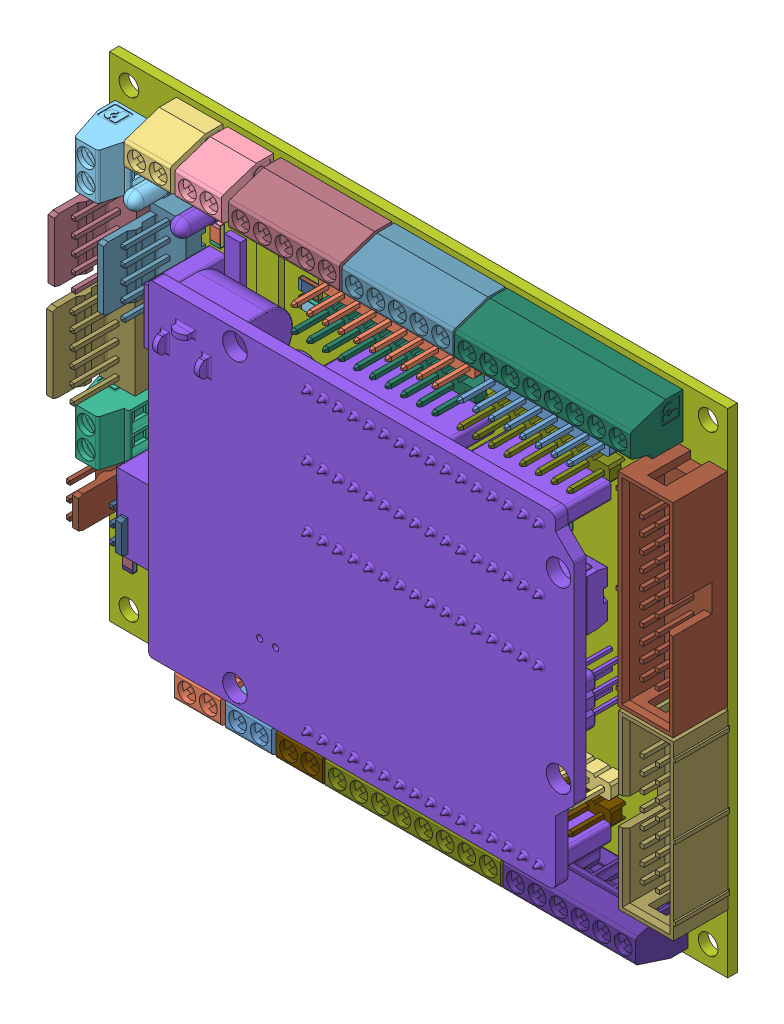
SolidWorks assembly Arduino Uno shield with Uno, configuration Standard. Lengths in mm.
Overall size (100.65 80.01 17.78).
190 component instances, 188 part files, 4 mates.
Components (placement in the parent):
- PPP5f08ec48b7509.stp-1: PPP5f08ec48b7509.stp [Standard] at origin size (100.65 80.01 15.26)
  - CAPRR500W50L750T250H650P002.stp-1: CAPRR500W50L750T250H650P002.stp [Standard] at (21.59 34.29 1.57) x (0 -1 0) z (0 0 1) size (7.5 2.5 6.5)
  - CAPRR500W50L750T250H650P001.stp-1: CAPRR500W50L750T250H650P001.stp [Standard] at (21.59 34.29 1.57) x (0 -1 0) z (0 0 1) size (0.5 0.5 6.5)
  - CAPRR500W50L750T250H650P.stp-1: CAPRR500W50L750T250H650P.stp [Standard] at (21.59 34.29 1.57) x (0 -1 0) z (0 0 1) size (0.5 0.5 6.5)
  - CAPRR500W50L750T250H650P003.stp-1: CAPRR500W50L750T250H650P003.stp [Standard] at (20.32 26.67 1.57) x (0 -1 0) z (0 0 1) size (7.5 2.5 6.5)
  - CAPRR500W50L750T250H650P004.stp-1: CAPRR500W50L750T250H650P004.stp [Standard] at (20.32 26.67 1.57) x (0 -1 0) z (0 0 1) size (0.5 0.5 6.5)
  - CAPRR500W50L750T250H650P005.stp-1: CAPRR500W50L750T250H650P005.stp [Standard] at (20.32 26.67 1.57) x (0 -1 0) z (0 0 1) size (0.5 0.5 6.5)
  - Component_1.stp-1: Component_1.stp [Standard] at (26.67 60.325 1.57) x (0 1 0) z (0 0 1) size (15.24 3.56 1)
  - SW3dPS-MELF_Cylinder5.stp-1: SW3dPS-MELF_Cylinder5.stp [Standard] at (33.02 13.208 1.57) x (0 1 0) z (0 0 1) size (0.5 2.5 2.5)
  - SW3dPS-MELF_Cylinder7.stp-1: SW3dPS-MELF_Cylinder7.stp [Standard] at (33.02 13.208 1.57) x (0 1 0) z (0 0 1) size (0.8 2.5 2.5)
  - SW3dPS-MELF_Board1.stp-1: SW3dPS-MELF_Board1.stp [Standard] at (33.02 13.208 1.57) x (0 1 0) z (0 0 1) size (1.7 0.01 0.01)
  - SW3dPS-MELF_Cylinder9.stp-1: SW3dPS-MELF_Cylinder9.stp [Standard] at (33.02 13.208 1.57) x (0 1 0) z (0 0 1) size (2.4 2.5 2.5)
  - SW3dPS-MELF_Cylinder8.stp-1: SW3dPS-MELF_Cylinder8.stp [Standard] at (33.02 13.208 1.57) x (0 1 0) z (0 0 1) size (0.5 2.5 2.5)
  - SW3dPS-MELF_Cylinder6.stp-1: SW3dPS-MELF_Cylinder6.stp [Standard] at (33.02 13.208 1.57) x (0 1 0) z (0 0 1) size (0.8 2.5 2.5)
  - SW3dPS-MELF_Cylinder010.stp-1: SW3dPS-MELF_Cylinder010.stp [Standard] at (41.275 13.208 1.57) x (0 1 0) z (0 0 1) size (0.5 2.5 2.5)
  - SW3dPS-MELF_Cylinder011.stp-1: SW3dPS-MELF_Cylinder011.stp [Standard] at (41.275 13.208 1.57) x (0 1 0) z (0 0 1) size (0.8 2.5 2.5)
  - SW3dPS-MELF_Board002.stp-1: SW3dPS-MELF_Board002.stp [Standard] at (41.275 13.208 1.57) x (0 1 0) z (0 0 1) size (1.7 0.01 0.01)
  - SW3dPS-MELF_Cylinder012.stp-1: SW3dPS-MELF_Cylinder012.stp [Standard] at (41.275 13.208 1.57) x (0 1 0) z (0 0 1) size (2.4 2.5 2.5)
  - SW3dPS-MELF_Cylinder013.stp-1: SW3dPS-MELF_Cylinder013.stp [Standard] at (41.275 13.208 1.57) x (0 1 0) z (0 0 1) size (0.5 2.5 2.5)
  - SW3dPS-MELF_Cylinder014.stp-1: SW3dPS-MELF_Cylinder014.stp [Standard] at (41.275 13.208 1.57) x (0 1 0) z (0 0 1) size (0.8 2.5 2.5)
  - SW3dPS-MELF_Cylinder015.stp-1: SW3dPS-MELF_Cylinder015.stp [Standard] at (24.765 13.208 1.57) x (0 1 0) z (0 0 1) size (0.5 2.5 2.5)
  - SW3dPS-MELF_Cylinder016.stp-1: SW3dPS-MELF_Cylinder016.stp [Standard] at (24.765 13.208 1.57) x (0 1 0) z (0 0 1) size (0.8 2.5 2.5)
  - SW3dPS-MELF_Board003.stp-1: SW3dPS-MELF_Board003.stp [Standard] at (24.765 13.208 1.57) x (0 1 0) z (0 0 1) size (1.7 0.01 0.01)
  - SW3dPS-MELF_Cylinder017.stp-1: SW3dPS-MELF_Cylinder017.stp [Standard] at (24.765 13.208 1.57) x (0 1 0) z (0 0 1) size (2.4 2.5 2.5)
  - SW3dPS-MELF_Cylinder018.stp-1: SW3dPS-MELF_Cylinder018.stp [Standard] at (24.765 13.208 1.57) x (0 1 0) z (0 0 1) size (0.5 2.5 2.5)
  - SW3dPS-MELF_Cylinder019.stp-1: SW3dPS-MELF_Cylinder019.stp [Standard] at (24.765 13.208 1.57) x (0 1 0) z (0 0 1) size (0.8 2.5 2.5)
  - Component_2.stp-1: Component_2.stp [Standard] at (20.955 59.69 1.57) x (0 -1 0) z (0 0 1) size (10.16 2.54 1)
  - Component_3.stp-1: Component_3.stp [Standard] at (20.32 43.815 1.57) x (-1 0 0) z (0 0 1) size (10.16 3.17 1)
  - =_[0_1_1_2].stp-1: =_[0_1_1_2].stp [Standard] at (10.795 24.13 1.57) x (0 -1 0) z (0 0 1) size (7.62 5.8 15.26)
  - =_[0_1_1_2]001.stp-1: =_[0_1_1_2]001.stp [Standard] at (3.81 24.13 1.57) x (0 -1 0) z (0 0 1) size (7.62 5.8 15.26)
  - =_[0_1_1_2]002.stp-1: =_[0_1_1_2]002.stp [Standard] at (4.445 44.45 1.57) x (0 1 0) z (0 0 1) size (15.24 5.8 15.26)
  - =_[0_1_1_2]003.stp-1: =_[0_1_1_2]003.stp [Standard] at (4.699 59.055 1.57) x (0 1 0) z (0 0 1) size (12.7 5.8 15.26)
  - =_[0_1_1_2]004.stp-1: =_[0_1_1_2]004.stp [Standard] at (12.7 59.055 1.57) x (0 1 0) z (0 0 1) size (12.7 5.8 15.26)
  - 1.stp-1: 1.stp [Standard] at (49.276 63.5 1.57) x (-1 0 0) z (0 0 1) size (25.4 2.5 11.2)
  - 1001.stp-1: 1001.stp [Standard] at (73.66 63.5 1.57) x (-1 0 0) z (0 0 1) size (20.32 2.5 11.2)
  - 1002.stp-1: 1002.stp [Standard] at (55.88 15.24 1.57) x (-1 0 0) z (0 0 1) size (20.32 2.5 11.2)
  - 1003.stp-1: 1003.stp [Standard] at (76.2 15.24 1.57) size (15.24 2.5 11.2)
  - 1004.stp-1: 1004.stp [Standard] at (73.66 67.31 1.57) x (-1 0 0) z (0 0 1) size (20.32 2.5 11.2)
  - 1005.stp-1: 1005.stp [Standard] at (49.276 67.31 1.57) x (-1 0 0) z (0 0 1) size (25.4 2.5 11.2)
  - 1006.stp-1: 1006.stp [Standard] at (76.2 19.05 1.57) size (15.24 2.5 11.2)
  - 1007.stp-1: 1007.stp [Standard] at (55.88 19.05 1.57) x (-1 0 0) z (0 0 1) size (20.32 2.5 11.2)
  - LEDRD254W000D310H620P002.stp-1: LEDRD254W000D310H620P002.stp [Standard] at (12.065 69.215 1.57) x (0 1 0) z (0 0 1) size (3.1 3.1 6.2)
  - LEDRD254W000D310H620P.stp-1: LEDRD254W000D310H620P.stp [Standard] at (12.065 69.215 1.57) x (0 1 0) z (0 0 1) size (0.38 0.38 6.2)
  - LEDRD254W000D310H620P001.stp-1: LEDRD254W000D310H620P001.stp [Standard] at (12.065 69.215 1.57) x (0 1 0) z (0 0 1) size (0.38 0.38 6.2)
  - LEDRD254W000D310H620P003.stp-1: LEDRD254W000D310H620P003.stp [Standard] at (19.685 69.215 1.57) x (0 1 0) z (0 0 1) size (3.1 3.1 6.2)
  - LEDRD254W000D310H620P004.stp-1: LEDRD254W000D310H620P004.stp [Standard] at (19.685 69.215 1.57) x (0 1 0) z (0 0 1) size (0.38 0.38 6.2)
  - LEDRD254W000D310H620P005.stp-1: LEDRD254W000D310H620P005.stp [Standard] at (19.685 69.215 1.57) x (0 1 0) z (0 0 1) size (0.38 0.38 6.2)
  - LEDRD254W000D310H620P006.stp-1: LEDRD254W000D310H620P006.stp [Standard] at (50.8 52.705 1.57) x (-1 0 0) z (0 0 1) size (3.1 3.1 6.2)
  - LEDRD254W000D310H620P007.stp-1: LEDRD254W000D310H620P007.stp [Standard] at (50.8 52.705 1.57) x (-1 0 0) z (0 0 1) size (0.38 0.38 6.2)
  - LEDRD254W000D310H620P008.stp-1: LEDRD254W000D310H620P008.stp [Standard] at (50.8 52.705 1.57) x (-1 0 0) z (0 0 1) size (0.38 0.38 6.2)
  - LEDRD254W000D310H620P009.stp-1: LEDRD254W000D310H620P009.stp [Standard] at (45.72 52.705 1.57) x (-1 0 0) z (0 0 1) size (3.1 3.1 6.2)
  - LEDRD254W000D310H620P010.stp-1: LEDRD254W000D310H620P010.stp [Standard] at (45.72 52.705 1.57) x (-1 0 0) z (0 0 1) size (0.38 0.38 6.2)
  - LEDRD254W000D310H620P011.stp-1: LEDRD254W000D310H620P011.stp [Standard] at (45.72 52.705 1.57) x (-1 0 0) z (0 0 1) size (0.38 0.38 6.2)
  - User_Library-TO263-3New_Extruded_2.stp-1: User_Library-TO263-3New_Extruded_2.stp [Standard] at (41.91 31.75 1.57) x (-1 0 0) z (0 0 1) size (1.4 1.53 0.51)
  - User_Library-TO263-3New_Extruded.stp-1: User_Library-TO263-3New_Extruded.stp [Standard] at (41.91 31.75 1.57) x (-1 0 0) z (0 0 1) size (1 5.77 3.36)
  - User_Library-TO263-3New_D2PACK.stp-1: User_Library-TO263-3New_D2PACK.stp [Standard] at (41.91 31.75 1.57) x (-1 0 0) z (0 0 1) size (10.41 15.85 4.61)
  - User_Library-TO263-3New_Extruded_003.stp-1: User_Library-TO263-3New_Extruded_003.stp [Standard] at (54.61 31.75 1.57) x (-1 0 0) z (0 0 1) size (1.4 1.53 0.51)
  - User_Library-TO263-3New_Extruded001.stp-1: User_Library-TO263-3New_Extruded001.stp [Standard] at (54.61 31.75 1.57) x (-1 0 0) z (0 0 1) size (1 5.77 3.36)
  - User_Library-TO263-3New_D2PACK001.stp-1: User_Library-TO263-3New_D2PACK001.stp [Standard] at (54.61 31.75 1.57) x (-1 0 0) z (0 0 1) size (10.41 15.85 4.61)
  - User_Library-TO263-3New_Extruded_004.stp-1: User_Library-TO263-3New_Extruded_004.stp [Standard] at (29.21 31.75 1.57) x (-1 0 0) z (0 0 1) size (1.4 1.53 0.51)
  - User_Library-TO263-3New_Extruded002.stp-1: User_Library-TO263-3New_Extruded002.stp [Standard] at (29.21 31.75 1.57) x (-1 0 0) z (0 0 1) size (1 5.77 3.36)
  - User_Library-TO263-3New_D2PACK002.stp-1: User_Library-TO263-3New_D2PACK002.stp [Standard] at (29.21 31.75 1.57) x (-1 0 0) z (0 0 1) size (10.41 15.85 4.61)
  - RESC3216X078.stp-1: RESC3216X078.stp [Standard] at (54.483 46.482 1.57) size (2.12 1.6 0.1)
  - RESC3216X079.stp-1: RESC3216X079.stp [Standard] at (54.483 46.482 1.57) size (3.06 1.6 0.56)
  - RESC3216X077.stp-1: RESC3216X077.stp [Standard] at (54.483 46.482 1.57) size (0.57 1.6 0.76)
  - RESC3216X080.stp-1: RESC3216X080.stp [Standard] at (54.483 46.482 1.57) size (2.12 1.6 0.1)
  - RESC3216X76.stp-1: RESC3216X76.stp [Standard] at (54.483 46.482 1.57) size (0.57 1.6 0.76)
  - RESC3216X081.stp-1: RESC3216X081.stp [Standard] at (41.91 46.355 1.57) size (2.12 1.6 0.1)
  - RESC3216X082.stp-1: RESC3216X082.stp [Standard] at (41.91 46.355 1.57) size (3.06 1.6 0.56)
  - RESC3216X083.stp-1: RESC3216X083.stp [Standard] at (41.91 46.355 1.57) size (0.57 1.6 0.76)
  - RESC3216X084.stp-1: RESC3216X084.stp [Standard] at (41.91 46.355 1.57) size (2.12 1.6 0.1)
  - RESC3216X085.stp-1: RESC3216X085.stp [Standard] at (41.91 46.355 1.57) size (0.57 1.6 0.76)
  - RESC3216X086.stp-1: RESC3216X086.stp [Standard] at (29.21 48.895 1.57) size (2.12 1.6 0.1)
  - RESC3216X087.stp-1: RESC3216X087.stp [Standard] at (29.21 48.895 1.57) size (3.06 1.6 0.56)
  - RESC3216X088.stp-1: RESC3216X088.stp [Standard] at (29.21 48.895 1.57) size (0.57 1.6 0.76)
  - RESC3216X089.stp-1: RESC3216X089.stp [Standard] at (29.21 48.895 1.57) size (2.12 1.6 0.1)
  - RESC3216X090.stp-1: RESC3216X090.stp [Standard] at (29.21 48.895 1.57) size (0.57 1.6 0.76)
  - RESC3216X091.stp-1: RESC3216X091.stp [Standard] at (33.02 60.96 1.57) size (2.12 1.6 0.1)
  - RESC3216X092.stp-1: RESC3216X092.stp [Standard] at (33.02 60.96 1.57) size (3.06 1.6 0.56)
  - RESC3216X093.stp-1: RESC3216X093.stp [Standard] at (33.02 60.96 1.57) size (0.57 1.6 0.76)
  - RESC3216X094.stp-1: RESC3216X094.stp [Standard] at (33.02 60.96 1.57) size (2.12 1.6 0.1)
  - RESC3216X095.stp-1: RESC3216X095.stp [Standard] at (33.02 60.96 1.57) size (0.57 1.6 0.76)
  - RESC3216X096.stp-1: RESC3216X096.stp [Standard] at (33.02 63.5 1.57) size (2.12 1.6 0.1)
  - RESC3216X097.stp-1: RESC3216X097.stp [Standard] at (33.02 63.5 1.57) size (3.06 1.6 0.56)
  - RESC3216X098.stp-1: RESC3216X098.stp [Standard] at (33.02 63.5 1.57) size (0.57 1.6 0.76)
  - RESC3216X099.stp-1: RESC3216X099.stp [Standard] at (33.02 63.5 1.57) size (2.12 1.6 0.1)
  - RESC3216X100.stp-1: RESC3216X100.stp [Standard] at (33.02 63.5 1.57) size (0.57 1.6 0.76)
  - RESC3216X101.stp-1: RESC3216X101.stp [Standard] at (15.875 69.215 1.57) x (0 -1 0) z (0 0 1) size (2.12 1.6 0.1)
  - RESC3216X102.stp-1: RESC3216X102.stp [Standard] at (15.875 69.215 1.57) x (0 -1 0) z (0 0 1) size (3.06 1.6 0.56)
  - RESC3216X103.stp-1: RESC3216X103.stp [Standard] at (15.875 69.215 1.57) x (0 -1 0) z (0 0 1) size (0.57 1.6 0.76)
  - RESC3216X104.stp-1: RESC3216X104.stp [Standard] at (15.875 69.215 1.57) x (0 -1 0) z (0 0 1) size (2.12 1.6 0.1)
  - RESC3216X105.stp-1: RESC3216X105.stp [Standard] at (15.875 69.215 1.57) x (0 -1 0) z (0 0 1) size (0.57 1.6 0.76)
  - RESC3216X106.stp-1: RESC3216X106.stp [Standard] at (17.907 63.627 1.57) x (0 1 0) z (0 0 1) size (2.12 1.6 0.1)
  - RESC3216X107.stp-1: RESC3216X107.stp [Standard] at (17.907 63.627 1.57) x (0 1 0) z (0 0 1) size (3.06 1.6 0.56)
  - RESC3216X108.stp-1: RESC3216X108.stp [Standard] at (17.907 63.627 1.57) x (0 1 0) z (0 0 1) size (0.57 1.6 0.76)
  - RESC3216X109.stp-1: RESC3216X109.stp [Standard] at (17.907 63.627 1.57) x (0 1 0) z (0 0 1) size (2.12 1.6 0.1)
  - RESC3216X110.stp-1: RESC3216X110.stp [Standard] at (17.907 63.627 1.57) x (0 1 0) z (0 0 1) size (0.57 1.6 0.76)
  - RESC3216X111.stp-1: RESC3216X111.stp [Standard] at (50.673 57.023 1.57) x (-1 0 0) z (0 0 1) size (2.12 1.6 0.1)
  - RESC3216X112.stp-1: RESC3216X112.stp [Standard] at (50.673 57.023 1.57) x (-1 0 0) z (0 0 1) size (3.06 1.6 0.56)
  - RESC3216X113.stp-1: RESC3216X113.stp [Standard] at (50.673 57.023 1.57) x (-1 0 0) z (0 0 1) size (0.57 1.6 0.76)
  - RESC3216X114.stp-1: RESC3216X114.stp [Standard] at (50.673 57.023 1.57) x (-1 0 0) z (0 0 1) size (2.12 1.6 0.1)
  - RESC3216X115.stp-1: RESC3216X115.stp [Standard] at (50.673 57.023 1.57) x (-1 0 0) z (0 0 1) size (0.57 1.6 0.76)
  - RESC3216X116.stp-1: RESC3216X116.stp [Standard] at (46.99 57.277 1.57) x (0 -1 0) z (0 0 1) size (2.12 1.6 0.1)
  - RESC3216X117.stp-1: RESC3216X117.stp [Standard] at (46.99 57.277 1.57) x (0 -1 0) z (0 0 1) size (3.06 1.6 0.56)
  - RESC3216X118.stp-1: RESC3216X118.stp [Standard] at (46.99 57.277 1.57) x (0 -1 0) z (0 0 1) size (0.57 1.6 0.76)
  - RESC3216X119.stp-1: RESC3216X119.stp [Standard] at (46.99 57.277 1.57) x (0 -1 0) z (0 0 1) size (2.12 1.6 0.1)
  - RESC3216X120.stp-1: RESC3216X120.stp [Standard] at (46.99 57.277 1.57) x (0 -1 0) z (0 0 1) size (0.57 1.6 0.76)
  - RESC3216X121.stp-1: RESC3216X121.stp [Standard] at (34.925 45.085 1.57) x (-1 0 0) z (0 0 1) size (2.12 1.6 0.1)
  - RESC3216X122.stp-1: RESC3216X122.stp [Standard] at (34.925 45.085 1.57) x (-1 0 0) z (0 0 1) size (3.06 1.6 0.56)
  - RESC3216X123.stp-1: RESC3216X123.stp [Standard] at (34.925 45.085 1.57) x (-1 0 0) z (0 0 1) size (0.57 1.6 0.76)
  - RESC3216X124.stp-1: RESC3216X124.stp [Standard] at (34.925 45.085 1.57) x (-1 0 0) z (0 0 1) size (2.12 1.6 0.1)
  - RESC3216X125.stp-1: RESC3216X125.stp [Standard] at (34.925 45.085 1.57) x (-1 0 0) z (0 0 1) size (0.57 1.6 0.76)
  - RESC3216X126.stp-1: RESC3216X126.stp [Standard] at (47.625 46.101 1.57) x (0 -1 0) z (0 0 1) size (2.12 1.6 0.1)
  - RESC3216X127.stp-1: RESC3216X127.stp [Standard] at (47.625 46.101 1.57) x (0 -1 0) z (0 0 1) size (3.06 1.6 0.56)
  - RESC3216X128.stp-1: RESC3216X128.stp [Standard] at (47.625 46.101 1.57) x (0 -1 0) z (0 0 1) size (0.57 1.6 0.76)
  - RESC3216X129.stp-1: RESC3216X129.stp [Standard] at (47.625 46.101 1.57) x (0 -1 0) z (0 0 1) size (2.12 1.6 0.1)
  - RESC3216X130.stp-1: RESC3216X130.stp [Standard] at (47.625 46.101 1.57) x (0 -1 0) z (0 0 1) size (0.57 1.6 0.76)
  - RESC3216X131.stp-1: RESC3216X131.stp [Standard] at (59.69 48.006 1.57) x (0 -1 0) z (0 0 1) size (2.12 1.6 0.1)
  - RESC3216X132.stp-1: RESC3216X132.stp [Standard] at (59.69 48.006 1.57) x (0 -1 0) z (0 0 1) size (3.06 1.6 0.56)
  - RESC3216X133.stp-1: RESC3216X133.stp [Standard] at (59.69 48.006 1.57) x (0 -1 0) z (0 0 1) size (0.57 1.6 0.76)
  - RESC3216X134.stp-1: RESC3216X134.stp [Standard] at (59.69 48.006 1.57) x (0 -1 0) z (0 0 1) size (2.12 1.6 0.1)
  - RESC3216X135.stp-1: RESC3216X135.stp [Standard] at (59.69 48.006 1.57) x (0 -1 0) z (0 0 1) size (0.57 1.6 0.76)
  - RESC2012X072.stp-1: RESC2012X072.stp [Standard] at (10.795 50.165 1.57) x (-1 0 0) z (0 0 1) size (1.2 1.25 0.1)
  - RESC2012X073.stp-1: RESC2012X073.stp [Standard] at (10.795 50.165 1.57) x (-1 0 0) z (0 0 1) size (1.8 1.25 0.5)
  - RESC2012X071.stp-1: RESC2012X071.stp [Standard] at (10.795 50.165 1.57) x (-1 0 0) z (0 0 1) size (0.4 1.25 0.7)
  - RESC2012X074.stp-1: RESC2012X074.stp [Standard] at (10.795 50.165 1.57) x (-1 0 0) z (0 0 1) size (1.2 1.25 0.1)
  - RESC2012X70.stp-1: RESC2012X70.stp [Standard] at (10.795 50.165 1.57) x (-1 0 0) z (0 0 1) size (0.4 1.25 0.7)
  - RESC2012X075.stp-1: RESC2012X075.stp [Standard] at (10.795 47.625 1.57) x (-1 0 0) z (0 0 1) size (1.2 1.25 0.1)
  - RESC2012X076.stp-1: RESC2012X076.stp [Standard] at (10.795 47.625 1.57) x (-1 0 0) z (0 0 1) size (1.8 1.25 0.5)
  - RESC2012X077.stp-1: RESC2012X077.stp [Standard] at (10.795 47.625 1.57) x (-1 0 0) z (0 0 1) size (0.4 1.25 0.7)
  - RESC2012X078.stp-1: RESC2012X078.stp [Standard] at (10.795 47.625 1.57) x (-1 0 0) z (0 0 1) size (1.2 1.25 0.1)
  - RESC2012X079.stp-1: RESC2012X079.stp [Standard] at (10.795 47.625 1.57) x (-1 0 0) z (0 0 1) size (0.4 1.25 0.7)
  - RESC2012X080.stp-1: RESC2012X080.stp [Standard] at (10.795 45.085 1.57) x (-1 0 0) z (0 0 1) size (1.2 1.25 0.1)
  - RESC2012X081.stp-1: RESC2012X081.stp [Standard] at (10.795 45.085 1.57) x (-1 0 0) z (0 0 1) size (1.8 1.25 0.5)
  - RESC2012X082.stp-1: RESC2012X082.stp [Standard] at (10.795 45.085 1.57) x (-1 0 0) z (0 0 1) size (0.4 1.25 0.7)
  - RESC2012X083.stp-1: RESC2012X083.stp [Standard] at (10.795 45.085 1.57) x (-1 0 0) z (0 0 1) size (1.2 1.25 0.1)
  - RESC2012X084.stp-1: RESC2012X084.stp [Standard] at (10.795 45.085 1.57) x (-1 0 0) z (0 0 1) size (0.4 1.25 0.7)
  - RESC2012X085.stp-1: RESC2012X085.stp [Standard] at (10.795 42.545 1.57) x (-1 0 0) z (0 0 1) size (1.2 1.25 0.1)
  - RESC2012X086.stp-1: RESC2012X086.stp [Standard] at (10.795 42.545 1.57) x (-1 0 0) z (0 0 1) size (1.8 1.25 0.5)
  - RESC2012X087.stp-1: RESC2012X087.stp [Standard] at (10.795 42.545 1.57) x (-1 0 0) z (0 0 1) size (0.4 1.25 0.7)
  - RESC2012X088.stp-1: RESC2012X088.stp [Standard] at (10.795 42.545 1.57) x (-1 0 0) z (0 0 1) size (1.2 1.25 0.1)
  - RESC2012X089.stp-1: RESC2012X089.stp [Standard] at (10.795 42.545 1.57) x (-1 0 0) z (0 0 1) size (0.4 1.25 0.7)
  - RESC2012X090.stp-1: RESC2012X090.stp [Standard] at (10.795 40.005 1.57) x (-1 0 0) z (0 0 1) size (1.2 1.25 0.1)
  - RESC2012X091.stp-1: RESC2012X091.stp [Standard] at (10.795 40.005 1.57) x (-1 0 0) z (0 0 1) size (1.8 1.25 0.5)
  - RESC2012X092.stp-1: RESC2012X092.stp [Standard] at (10.795 40.005 1.57) x (-1 0 0) z (0 0 1) size (0.4 1.25 0.7)
  - RESC2012X093.stp-1: RESC2012X093.stp [Standard] at (10.795 40.005 1.57) x (-1 0 0) z (0 0 1) size (1.2 1.25 0.1)
  - RESC2012X094.stp-1: RESC2012X094.stp [Standard] at (10.795 40.005 1.57) x (-1 0 0) z (0 0 1) size (0.4 1.25 0.7)
  - RESC2012X095.stp-1: RESC2012X095.stp [Standard] at (10.795 37.465 1.57) x (-1 0 0) z (0 0 1) size (1.2 1.25 0.1)
  - RESC2012X096.stp-1: RESC2012X096.stp [Standard] at (10.795 37.465 1.57) x (-1 0 0) z (0 0 1) size (1.8 1.25 0.5)
  - RESC2012X097.stp-1: RESC2012X097.stp [Standard] at (10.795 37.465 1.57) x (-1 0 0) z (0 0 1) size (0.4 1.25 0.7)
  - RESC2012X098.stp-1: RESC2012X098.stp [Standard] at (10.795 37.465 1.57) x (-1 0 0) z (0 0 1) size (1.2 1.25 0.1)
  - RESC2012X099.stp-1: RESC2012X099.stp [Standard] at (10.795 37.465 1.57) x (-1 0 0) z (0 0 1) size (0.4 1.25 0.7)
  - RESC3216X136.stp-1: RESC3216X136.stp [Standard] at (64.135 32.639 1.57) x (0 1 0) z (0 0 1) size (2.12 1.6 0.1)
  - RESC3216X137.stp-1: RESC3216X137.stp [Standard] at (64.135 32.639 1.57) x (0 1 0) z (0 0 1) size (3.06 1.6 0.56)
  - RESC3216X138.stp-1: RESC3216X138.stp [Standard] at (64.135 32.639 1.57) x (0 1 0) z (0 0 1) size (0.57 1.6 0.76)
  - RESC3216X139.stp-1: RESC3216X139.stp [Standard] at (64.135 32.639 1.57) x (0 1 0) z (0 0 1) size (2.12 1.6 0.1)
  - RESC3216X140.stp-1: RESC3216X140.stp [Standard] at (64.135 32.639 1.57) x (0 1 0) z (0 0 1) size (0.57 1.6 0.76)
  - RESC3216X141.stp-1: RESC3216X141.stp [Standard] at (3.683 10.795 1.57) x (0 1 0) z (0 0 1) size (2.12 1.6 0.1)
  - RESC3216X142.stp-1: RESC3216X142.stp [Standard] at (3.683 10.795 1.57) x (0 1 0) z (0 0 1) size (3.06 1.6 0.56)
  - RESC3216X143.stp-1: RESC3216X143.stp [Standard] at (3.683 10.795 1.57) x (0 1 0) z (0 0 1) size (0.57 1.6 0.76)
  - RESC3216X144.stp-1: RESC3216X144.stp [Standard] at (3.683 10.795 1.57) x (0 1 0) z (0 0 1) size (2.12 1.6 0.1)
  - RESC3216X145.stp-1: RESC3216X145.stp [Standard] at (3.683 10.795 1.57) x (0 1 0) z (0 0 1) size (0.57 1.6 0.76)
  - RESC3216X146.stp-1: RESC3216X146.stp [Standard] at (74.422 51.943 1.57) x (0 -1 0) z (0 0 1) size (2.12 1.6 0.1)
  - RESC3216X147.stp-1: RESC3216X147.stp [Standard] at (74.422 51.943 1.57) x (0 -1 0) z (0 0 1) size (3.06 1.6 0.56)
  - RESC3216X148.stp-1: RESC3216X148.stp [Standard] at (74.422 51.943 1.57) x (0 -1 0) z (0 0 1) size (0.57 1.6 0.76)
  - RESC3216X149.stp-1: RESC3216X149.stp [Standard] at (74.422 51.943 1.57) x (0 -1 0) z (0 0 1) size (2.12 1.6 0.1)
  - RESC3216X150.stp-1: RESC3216X150.stp [Standard] at (74.422 51.943 1.57) x (0 -1 0) z (0 0 1) size (0.57 1.6 0.76)
  - RESC3216X151.stp-1: RESC3216X151.stp [Standard] at (3.683 17.272 1.57) x (0 1 0) z (0 0 1) size (2.12 1.6 0.1)
  - RESC3216X152.stp-1: RESC3216X152.stp [Standard] at (3.683 17.272 1.57) x (0 1 0) z (0 0 1) size (3.06 1.6 0.56)
  - RESC3216X153.stp-1: RESC3216X153.stp [Standard] at (3.683 17.272 1.57) x (0 1 0) z (0 0 1) size (0.57 1.6 0.76)
  - RESC3216X154.stp-1: RESC3216X154.stp [Standard] at (3.683 17.272 1.57) x (0 1 0) z (0 0 1) size (2.12 1.6 0.1)
  - RESC3216X155.stp-1: RESC3216X155.stp [Standard] at (3.683 17.272 1.57) x (0 1 0) z (0 0 1) size (0.57 1.6 0.76)
  - Component_4.stp-1: Component_4.stp [Standard] at (11.684 10.287 1.57) size (2 2 1)
  - User_Library-BH-10...64.stp-1: User_Library-BH-10...64.stp [Standard] at (95.885 54.61 1.57) x (0 1 0) z (0 0 1) size (33.06 9.2 12.14)
  - User_Library-BH-10...065.stp-1: User_Library-BH-10...065.stp [Standard] at (95.885 23.495 1.57) x (0 -1 0) z (0 0 1) size (27.98 9.2 12.14)
  - mkds_1-5-3.5_mkds_1-5-3.5;mkds_1-5-3.5.stp-1: mkds_1-5-3.5_mkds_1-5-3.5;mkds_1-5-3.5.stp [Standard] at (36.83 75.565 1.57) size (18 7.3 12)
  - mkds_1-5-3.5_mkds_1-5-3.5;mkds_1-5-3.006.stp-1: mkds_1-5-3.5_mkds_1-5-3.5;mkds_1-5-3.006.stp [Standard] at (55.245 75.565 1.57) size (18 7.3 12)
  - mkds_1-8-3.5_mkds_1-8-3.5;mkds_1-8-3.5.stp-1: mkds_1-8-3.5_mkds_1-8-3.5;mkds_1-8-3.5.stp [Standard] at (78.74 75.565 1.57) size (28.5 7.3 12)
  - mkds_1-8-3.5_mkds_1-8-3.5;mkds_1-8-3.006.stp-1: mkds_1-8-3.5_mkds_1-8-3.5;mkds_1-8-3.006.stp [Standard] at (57.785 4.445 1.57) x (-1 0 0) z (0 0 1) size (28.5 7.3 12)
  - mkds_1-6-3.5_mkds_1-6-3.5;mkds_1-6-3.5.stp-1: mkds_1-6-3.5_mkds_1-6-3.5;mkds_1-6-3.5.stp [Standard] at (83.185 4.445 1.57) x (-1 0 0) z (0 0 1) size (21.5 7.3 12)
  - mkds_1-2-3.5_mkds_1-2-3.5;mkds_1-2-3.5.stp-1: mkds_1-2-3.5_mkds_1-2-3.5;mkds_1-2-3.5.stp [Standard] at (39.37 4.445 1.57) x (-1 0 0) z (0 0 1) size (7.5 7.3 12)
  - mkds_1-2-3.5_mkds_1-2-3.5;mkds_1-2-3.006.stp-1: mkds_1-2-3.5_mkds_1-2-3.5;mkds_1-2-3.006.stp [Standard] at (31.115 4.445 1.57) x (-1 0 0) z (0 0 1) size (7.5 7.3 12)
  - mkds_1-2-3.5_mkds_1-2-3.5;mkds_1-2-3.007.stp-1: mkds_1-2-3.5_mkds_1-2-3.5;mkds_1-2-3.007.stp [Standard] at (22.86 4.445 1.57) x (-1 0 0) z (0 0 1) size (7.5 7.3 12)
  - mkds_1-2-3.5_mkds_1-2-3.5;mkds_1-2-3.008.stp-1: mkds_1-2-3.5_mkds_1-2-3.5;mkds_1-2-3.008.stp [Standard] at (14.605 75.565 1.57) size (7.5 7.3 12)
  - mkds_1-2-3.5_mkds_1-2-3.5;mkds_1-2-3.009.stp-1: mkds_1-2-3.5_mkds_1-2-3.5;mkds_1-2-3.009.stp [Standard] at (22.86 75.565 1.57) size (7.5 7.3 12)
  - mkds_1-2-3.5_mkds_1-2-3.5;mkds_1-2-3.010.stp-1: mkds_1-2-3.5_mkds_1-2-3.5;mkds_1-2-3.010.stp [Standard] at (4.445 69.85 1.57) x (0 1 0) z (0 0 1) size (7.5 7.3 12)
  - mkds_1-2-3.5_mkds_1-2-3.5;mkds_1-2-3.011.stp-1: mkds_1-2-3.5_mkds_1-2-3.5;mkds_1-2-3.011.stp [Standard] at (4.445 32.385 1.57) x (0 1 0) z (0 0 1) size (7.5 7.3 12)
  - Component_Component.stp-1: Component_Component.stp [Standard] at origin size (100.33 80.01 1.57)
- arduino uno-2: arduino uno [Default] at (52.02 37.3929 14.21) x (1 0 0) z (0 1 0) size (76.5 14.6 53)
- kkkrr-2: kkkrr [Default] at (132.8181 -85.8824 -60.2258) x (0.934285 0.356528 0) z (0 0 1) (suppressed, hidden)
Mates (geometry in assembly coordinates):
- Deckungsgleich2: coincident anti-aligned: plane of PPP5f08ec48b7509.stp-1/1006.stp-1 through (69.95 19.0531 4.11) normal (0 0 1); plane of arduino uno-2 through (52.02 37.3929 4.11) normal (0 0 -1)
- Deckungsgleich3: coincident aligned: line of PPP5f08ec48b7509.stp-1/1006.stp-1 through (83.92 19.9013 4.11) axis (0 -1 0); line of arduino uno-2 through (83.92 14.2929 4.11) axis (0 -1 0)
- Concentric5: concentric aligned: circle of PPP5f08ec48b7509.stp-1/Component_Component.stp-1; circle of kkk-2/base-1
- Concentric6: concentric aligned: circle of PPP5f08ec48b7509.stp-1/Component_Component.stp-1; circle of kkk-2/base-1
